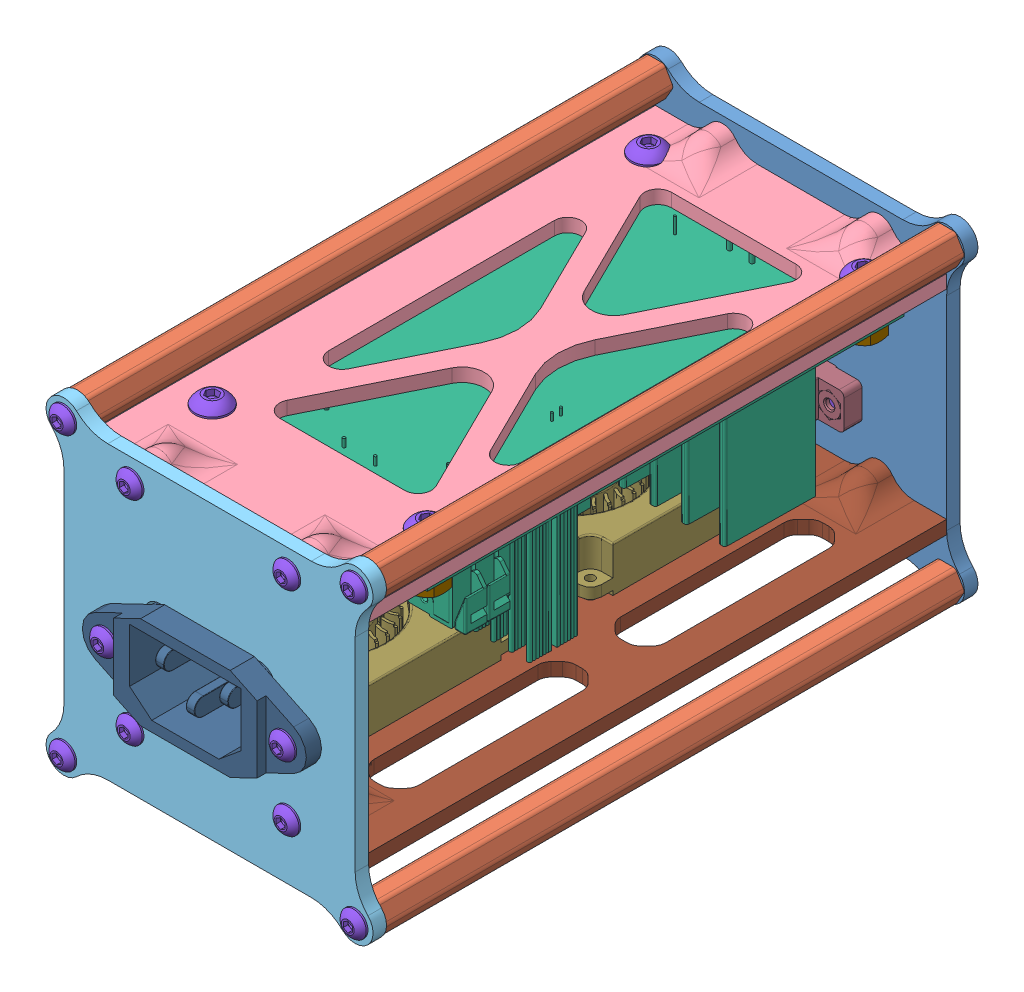
SolidWorks assembly ASM-box-changer-power, configuration По умолчанию. Lengths in mm.
Overall size (73 73 142.05).
63 component instances, 13 part files, 116 mates.
Components (placement in the parent):
- 65-65-3-1: 65-65-3 [По умолчанию] at origin size (73 73 3)
- stoyka-7-129-1: stoyka-7-129 [По умолчанию] at (-32.5 -32.5 3) size (7.77 7 129)
- M3 insert nut.step-1: M3 insert nut.step [По умолчанию] at (-32.5 -32.5 6.1) size (4.49 4.48 6.21)
- M3 insert nut.step-2: M3 insert nut.step [По умолчанию] at (-32.5 -32.5 128.9) size (4.49 4.48 6.21)
- M3 insert nut.step-3: M3 insert nut.step [По умолчанию] at (-32.5 32.5 128.9) size (4.49 4.48 6.21)
- M3 insert nut.step-4: M3 insert nut.step [По умолчанию] at (32.5 -32.5 128.9) size (4.49 4.48 6.21)
- M3 insert nut.step-5: M3 insert nut.step [По умолчанию] at (32.5 32.5 128.9) size (4.49 4.48 6.21)
- M3 insert nut.step-6: M3 insert nut.step [По умолчанию] at (-32.5 32.5 6.1) size (4.49 4.48 6.21)
- M3 insert nut.step-7: M3 insert nut.step [По умолчанию] at (32.5 -32.5 6.1) size (4.49 4.48 6.21)
- M3 insert nut.step-8: M3 insert nut.step [По умолчанию] at (32.5 32.5 6.1) size (4.49 4.48 6.21)
- stoyka-7-129-2: stoyka-7-129 [По умолчанию] at (-32.5 32.5 3) size (7.77 7 129)
- stoyka-7-129-3: stoyka-7-129 [По умолчанию] at (32.5 -32.5 3) size (7.77 7 129)
- stoyka-7-129-4: stoyka-7-129 [По умолчанию] at (32.5 32.5 3) size (7.77 7 129)
- level-0-1: level-0 [По умолчанию] at (0 27 67.5) x (0 0 1) z (0 -1 0) size (129 65 7)
- M3 insert nut.step-9: M3 insert nut.step [По умолчанию] at (-17.5 27.5 6.1) size (4.49 4.48 6.21)
- M3 insert nut.step-10: M3 insert nut.step [По умолчанию] at (17.5 27.5 6.1) size (4.49 4.48 6.21)
- M3 insert nut.step-11: M3 insert nut.step [По умолчанию] at (17.5 27.5 128.9) size (4.49 4.48 6.21)
- M3 insert nut.step-12: M3 insert nut.step [По умолчанию] at (-17.5 27.5 128.9) size (4.49 4.48 6.21)
- 65-65-3-down-1: 65-65-3-down [По умолчанию] at (0 0 132) size (73 73 3)
- WX-DC2412-1: WX-DC2412 [По умолчанию] at (0 21 61.7) x (0 0 -1) z (0 -1 0) size (106.4 57 32.5)
- 4-8-3-1: 4-8-3 [По умолчанию] at (24 21 110.4) x (0.995679 0 0.09286) z (-0.09286 0 0.995679) size (8 3 8)
- 4-8-3-2: 4-8-3 [По умолчанию] at (24 21 13) size (8 3 8)
- 4-8-3-3: 4-8-3 [По умолчанию] at (-24 21 110.4) size (8 3 8)
- 4-8-3-4: 4-8-3 [По умолчанию] at (-24 21 13) size (8 3 8)
- socket button head screw_iso-1: socket button head screw_iso [ISO 7380 - M3 x 8 - 8N] at (17.5 27.5 136.65) x (0 0 -1) z (1 0 0) size (9.65 5.7 5.7)
- socket button head screw_iso-2: socket button head screw_iso [ISO 7380 - M3 x 8 - 8N] at (-17.5 27.5 136.65) x (0 0 -1) z (1 0 0) size (9.65 5.7 5.7)
- socket button head screw_iso-3: socket button head screw_iso [ISO 7380 - M3 x 8 - 8N] at (-32.5 32.5 136.65) x (0 0 -1) z (1 0 0) size (9.65 5.7 5.7)
- socket button head screw_iso-4: socket button head screw_iso [ISO 7380 - M3 x 8 - 8N] at (32.5 32.5 136.65) x (0 0 -1) z (1 0 0) size (9.65 5.7 5.7)
- socket button head screw_iso-5: socket button head screw_iso [ISO 7380 - M3 x 8 - 8N] at (17.5 27.5 -1.65) x (0 0 1) z (-1 0 0) size (9.65 5.7 5.7)
- socket button head screw_iso-6: socket button head screw_iso [ISO 7380 - M3 x 8 - 8N] at (32.5 32.5 -1.65) x (0 0 1) z (-1 0 0) size (9.65 5.7 5.7)
- socket button head screw_iso-7: socket button head screw_iso [ISO 7380 - M3 x 8 - 8N] at (-17.5 27.5 -1.65) x (0 0 1) z (-1 0 0) size (9.65 5.7 5.7)
- socket button head screw_iso-8: socket button head screw_iso [ISO 7380 - M3 x 8 - 8N] at (-32.5 32.5 -1.65) x (0 0 1) z (-1 0 0) size (9.65 5.7 5.7)
- socket button head screw_iso-9: socket button head screw_iso [ISO 7380 - M4 x 12 - 12N] at (24 29.2 110.4) x (0 -1 0) z (0 0 1) size (14.2 7.6 7.6)
- socket button head screw_iso-10: socket button head screw_iso [ISO 7380 - M4 x 12 - 12N] at (24 29.2 13) x (0 -1 0) z (0 0 1) size (14.2 7.6 7.6)
- socket button head screw_iso-11: socket button head screw_iso [ISO 7380 - M4 x 12 - 12N] at (-24 29.2 13) x (0 -1 0) z (0 0 1) size (14.2 7.6 7.6)
- socket button head screw_iso-12: socket button head screw_iso [ISO 7380 - M4 x 12 - 12N] at (-24 29.2 110.4) x (0 -1 0) z (0 0 1) size (14.2 7.6 7.6)
- hex nut style 1 gradeab_iso-1: hex nut style 1 gradeab_iso [ISO - 4032 - M4 - D - N] at (24 16.3 110.4) x (1 0 0) z (0 -1 0) size (7 8.08 3.2)
- hex nut style 1 gradeab_iso-2: hex nut style 1 gradeab_iso [ISO - 4032 - M4 - D - N] at (24 16.28 13) x (1 0 0) z (0 -1 0) size (7 8.08 3.2)
- hex nut style 1 gradeab_iso-3: hex nut style 1 gradeab_iso [ISO - 4032 - M4 - D - N] at (-24 16.3 13) x (1 0 0) z (0 -1 0) size (7 8.08 3.2)
- hex nut style 1 gradeab_iso-4: hex nut style 1 gradeab_iso [ISO - 4032 - M4 - D - N] at (-24 16.28 110.4) x (1 0 0) z (0 -1 0) size (7 8.08 3.2)
- interlock.stp-1: interlock.stp [По умолчанию] at (0 -2.6153 135) size (50 20.7 27.56)
- level-1-1: level-1 [По умолчанию] at (0 -20.5 67.5) x (0 0 1) z (0 -1 0) size (129 65 7)
- 4010 turbo fan v3-1: 4010 turbo fan v3 [По умолчанию] at (-10 -20.5 40) x (1 0 0) z (0 1 0) size (40 40 10)
- 4010 turbo fan v3-2: 4010 turbo fan v3 [По умолчанию] at (-10 -20.5 95) x (1 0 0) z (0 1 0) size (40 40 10)
- M3 insert nut.step-13: M3 insert nut.step [По умолчанию] at (-17.5 -20 128.9) size (4.49 4.48 6.21)
- M3 insert nut.step-14: M3 insert nut.step [По умолчанию] at (17.5 -20 128.9) size (4.49 4.48 6.21)
- M3 insert nut.step-15: M3 insert nut.step [По умолчанию] at (-17.5 -20 6.1) size (4.49 4.48 6.21)
- M3 insert nut.step-16: M3 insert nut.step [По умолчанию] at (17.5 -20 6.1) size (4.49 4.48 6.21)
- socket button head screw_iso-13: socket button head screw_iso [ISO 7380 - M3 x 12 - 12N] at (-20 -2.6153 140.05) x (0 0 -1) z (1 0 0) size (13.65 5.7 5.7)
- socket button head screw_iso-14: socket button head screw_iso [ISO 7380 - M3 x 12 - 12N] at (20 -2.6153 140.05) x (0 0 -1) z (1 0 0) size (13.65 5.7 5.7)
- socket button head screw_iso-17: socket button head screw_iso [ISO 7380 - M3 x 8 - 8N] at (-17.5 -20 136.65) x (0 0 -1) z (1 0 0) size (9.65 5.7 5.7)
- socket button head screw_iso-18: socket button head screw_iso [ISO 7380 - M3 x 8 - 8N] at (17.5 -20 136.65) x (0 0 -1) z (1 0 0) size (9.65 5.7 5.7)
- socket button head screw_iso-19: socket button head screw_iso [ISO 7380 - M3 x 8 - 8N] at (-32.5 -32.5 136.65) x (0 0 -1) z (1 0 0) size (9.65 5.7 5.7)
- socket button head screw_iso-20: socket button head screw_iso [ISO 7380 - M3 x 8 - 8N] at (32.5 -32.5 136.65) x (0 0 -1) z (1 0 0) size (9.65 5.7 5.7)
- socket button head screw_iso-21: socket button head screw_iso [ISO 7380 - M3 x 8 - 8N] at (-32.5 -32.5 -1.65) x (0 0 1) z (-1 0 0) size (9.65 5.7 5.7)
- socket button head screw_iso-22: socket button head screw_iso [ISO 7380 - M3 x 8 - 8N] at (32.5 -32.5 -1.65) x (0 0 1) z (-1 0 0) size (9.65 5.7 5.7)
- hex nut style 1 gradeab_iso-5: hex nut style 1 gradeab_iso [ISO - 4032 - M3 - D - N] at (-20 -2.6153 129.6) x (0.923728 0.383049 0) z (0 0 -1) size (5.5 6.35 2.4)
- hex nut style 1 gradeab_iso-6: hex nut style 1 gradeab_iso [ISO - 4032 - M3 - D - N] at (20 -2.6153 129.6) x (0.923728 0.383049 0) z (0 0 -1) size (5.5 6.35 2.4)
- socket button head screw_iso-23: socket button head screw_iso [ISO 7380 - M3 x 8 - 8N] at (17.5 -20 -1.65) x (0 0 1) z (-1 0 0) size (9.65 5.7 5.7)
- socket button head screw_iso-24: socket button head screw_iso [ISO 7380 - M3 x 8 - 8N] at (-17.5 -20 -1.65) x (0 0 1) z (-1 0 0) size (9.65 5.7 5.7)
- XT60E-M-1: XT60E-M [00] at (0 -7.5 0) x (1 0 0) z (0 -1 0) size (27.2 16.65 9.1)
- socket button head screw_iso-27: socket button head screw_iso [ISO 7380 - M3 x 6 - 6N] at (10.3 -7.5 -1.65) x (0 0 1) z (-1 0 0) size (7.65 5.7 5.7)
- socket button head screw_iso-28: socket button head screw_iso [ISO 7380 - M3 x 6 - 6N] at (-10.3 -7.5 -1.65) x (0 0 1) z (-1 0 0) size (7.65 5.7 5.7)
Mates (geometry in assembly coordinates):
- Концентричный1: concentric anti-aligned: cylinder of 65-65-3-1 through (-32.5 -32.5 3) axis (0 0 -1) radius 1.625; cylinder of stoyka-7-129-1 through (-32.5 -32.5 126) axis (0 0 1) radius 2.25
- Параллельность1: parallel aligned: plane of 65-65-3-1 through (0 -32.5 3) normal (0 -1 0); plane of stoyka-7-129-1 through (-33.9434 -36 132) normal (0 -1 0)
- Концентричный2: concentric aligned: cylinder of stoyka-7-129-1 through (-32.5 -32.5 9) axis (0 0 -1) radius 2.25; cylinder of M3 insert nut.step-1 through (-32.5 -32.5 9.2) axis (0 0 -1) radius 2
- Совпадение2: coincident aligned: plane of stoyka-7-129-1 through (-35.3868 -32.5 3) normal (0 0 -1); plane of M3 insert nut.step-1 through (-32.5 -32.5 3) normal (0 0 -1)
- Концентричный3: concentric anti-aligned: cylinder of stoyka-7-129-1 through (-32.5 -32.5 126) axis (0 0 1) radius 2.25; cylinder of M3 insert nut.step-2 through (-32.5 -32.5 132) axis (0 0 -1) radius 2
- Совпадение3: coincident aligned: plane of stoyka-7-129-1 through (-35.3868 -32.5 132) normal (0 0 1); plane of M3 insert nut.step-2 through (-32.5 -32.5 132) normal (0 0 1)
- Совпадение4: coincident anti-aligned: plane of 65-65-3-1 through (0 0 3) normal (0 0 1); plane of stoyka-7-129-1 through (-35.3868 -32.5 3) normal (0 0 -1)
- Концентричный4: concentric aligned: cylinder of level-0-1 through (-17.5 27.5 9) axis (0 0 -1) radius 2; cylinder of M3 insert nut.step-9 through (-17.5 27.5 9.2) axis (0 0 -1) radius 2
- Совпадение5: coincident aligned: plane of level-0-1 through (32.5 24 3) normal (0 0 -1); plane of M3 insert nut.step-9 through (-17.5 27.5 3) normal (0 0 -1)
- Концентричный5: concentric aligned: cylinder of level-0-1 through (17.5 27.5 9) axis (0 0 -1) radius 2; cylinder of M3 insert nut.step-10 through (17.5 27.5 9.2) axis (0 0 -1) radius 2
- Совпадение6: coincident aligned: plane of level-0-1 through (32.5 24 3) normal (0 0 -1); plane of M3 insert nut.step-10 through (17.5 27.5 3) normal (0 0 -1)
- Концентричный6: concentric anti-aligned: cylinder of level-0-1 through (17.5 27.5 126) axis (0 0 1) radius 2; cylinder of M3 insert nut.step-11 through (17.5 27.5 132) axis (0 0 -1) radius 2
- Совпадение8: coincident aligned: plane of level-0-1 through (32.5 24 132) normal (0 0 1); plane of M3 insert nut.step-11 through (17.5 27.5 132) normal (0 0 1)
- Концентричный7: concentric anti-aligned: cylinder of level-0-1 through (-17.5 27.5 126) axis (0 0 1) radius 2; cylinder of M3 insert nut.step-12 through (-17.5 27.5 132) axis (0 0 -1) radius 2
- Совпадение9: coincident aligned: plane of level-0-1 through (32.5 24 132) normal (0 0 1); plane of M3 insert nut.step-12 through (-17.5 27.5 132) normal (0 0 1)
- Совпадение10: coincident aligned: axis of M3 insert nut.step-5 through (32.5 32.5 130.25) axis (0 0 -1); line of 65-65-3-down-1 through (32.5 32.5 135) axis (0 0 -1)
- Параллельность2: parallel aligned: plane of 65-65-3-1 through (0 32.5 3) normal (0 1 0); plane of 65-65-3-down-1 through (0 32.5 135) normal (0 1 0)
- Совпадение12: coincident anti-aligned: plane of stoyka-7-129-4 through (29.6132 32.5 132) normal (0 0 1); plane of 65-65-3-down-1 through (0 0 132) normal (0 0 -1)
- Совпадение13: coincident anti-aligned: line of 65-65-3-1 through (17.5 27.5 3) axis (0 0 -1); line of M3 insert nut.step-10 through (17.5 27.5 3.0576) axis (0 0 1)
- Совпадение14: coincident aligned: line of 65-65-3-1 through (-17.5 27.5 3) axis (0 0 -1); line of level-0-1 through (-17.5 27.5 6.2156) axis (0 0 -1)
- Совпадение15: coincident anti-aligned: plane of 65-65-3-1 through (0 0 3) normal (0 0 1); plane of level-0-1 through (32.5 24 3) normal (0 0 -1)
- Концентричный8: concentric anti-aligned: cylinder of level-0-1 through (24 34 13) axis (0 -1 0) radius 2.25; cylinder of WX-DC2412-1 through (24 19.5 13) axis (0 1 0) radius 2
- Концентричный9: concentric aligned: cylinder of level-0-1 through (24 34 110.4) axis (0 -1 0) radius 2.25; cylinder of WX-DC2412-1 through (24 19.5 110.4) axis (0 -1 0) radius 2
- Концентричный10: concentric aligned: cylinder of level-0-1 through (24 34 13) axis (0 -1 0) radius 2.25; cylinder of 4-8-3-2 through (24 24 13) axis (0 -1 0) radius 2.25
- Концентричный11: concentric anti-aligned: cylinder of WX-DC2412-1 through (24 19.5 13) axis (0 1 0) radius 2; cylinder of 4-8-3-2 through (24 24 13) axis (0 -1 0) radius 2.25
- Совпадение16: coincident anti-aligned: plane of WX-DC2412-1 through (0 21 61.7) normal (0 1 0); plane of 4-8-3-2 through (24 21 13) normal (0 -1 0)
- Концентричный12: concentric anti-aligned: cylinder of WX-DC2412-1 through (24 19.5 110.4) axis (0 -1 0) radius 2; circle of 4-8-3-1
- Совпадение17: coincident anti-aligned: plane of WX-DC2412-1 through (0 21 61.7) normal (0 1 0); plane of 4-8-3-1 through (24 21 110.4) normal (0 -1 0)
- Концентричный13: concentric aligned: cylinder of level-0-1 through (-24 34 110.4) axis (0 -1 0) radius 2.25; cylinder of 4-8-3-3 through (-24 24 110.4) axis (0 -1 0) radius 2.25
- Совпадение18: coincident anti-aligned: plane of WX-DC2412-1 through (0 21 61.7) normal (0 1 0); plane of 4-8-3-3 through (-24 21 110.4) normal (0 -1 0)
- Концентричный14: concentric aligned: cylinder of WX-DC2412-1 through (-24 19.5 13) axis (0 -1 0) radius 2; cylinder of 4-8-3-4 through (-24 24 13) axis (0 -1 0) radius 2.25
- Совпадение19: coincident anti-aligned: plane of WX-DC2412-1 through (0 21 61.7) normal (0 1 0); plane of 4-8-3-4 through (-24 21 13) normal (0 -1 0)
- Совпадение20: coincident anti-aligned: plane of level-0-1 through (0 24 67.5) normal (0 -1 0); plane of 4-8-3-4 through (-24 24 13) normal (0 1 0)
- Концентричный15: concentric anti-aligned: cylinder of 65-65-3-down-1 through (17.5 27.5 142) axis (0 0 -1) radius 1.75; cylinder of socket button head screw_iso-1 through (17.5 27.5 136.65) axis (0 0 1) radius 2.85
- Совпадение21: coincident anti-aligned: plane of 65-65-3-down-1 through (0 0 135) normal (0 0 1); plane of socket button head screw_iso-1 through (17.5 29 135) normal (0 0 -1)
- Концентричный16: concentric anti-aligned: cylinder of 65-65-3-down-1 through (-17.5 27.5 142) axis (0 0 -1) radius 1.75; cylinder of socket button head screw_iso-2 through (-17.5 27.5 136.65) axis (0 0 1) radius 2.85
- Совпадение22: coincident anti-aligned: plane of 65-65-3-down-1 through (0 0 135) normal (0 0 1); plane of socket button head screw_iso-2 through (-17.5 29 135) normal (0 0 -1)
- Концентричный17: concentric anti-aligned: cylinder of 65-65-3-down-1 through (-32.5 32.5 135) axis (0 0 -1) radius 1.625; cylinder of socket button head screw_iso-3 through (-32.5 32.5 136.65) axis (0 0 1) radius 2.85
- Совпадение23: coincident anti-aligned: plane of 65-65-3-down-1 through (0 0 135) normal (0 0 1); plane of socket button head screw_iso-3 through (-32.5 34 135) normal (0 0 -1)
- Концентричный18: concentric anti-aligned: cylinder of 65-65-3-down-1 through (32.5 32.5 135) axis (0 0 -1) radius 4; cylinder of socket button head screw_iso-4 through (32.5 32.5 136.65) axis (0 0 1) radius 2.85
- Совпадение24: coincident anti-aligned: plane of 65-65-3-down-1 through (0 0 135) normal (0 0 1); plane of socket button head screw_iso-4 through (32.5 34 135) normal (0 0 -1)
- Концентричный19: concentric aligned: cylinder of 65-65-3-1 through (17.5 27.5 10) axis (0 0 -1) radius 1.75; cylinder of socket button head screw_iso-5 through (17.5 27.5 -1.65) axis (0 0 -1) radius 2.85
- Совпадение25: coincident anti-aligned: plane of 65-65-3-1 through (0 0 0) normal (0 0 -1); plane of socket button head screw_iso-5 through (17.5 29 0) normal (0 0 1)
- Концентричный20: concentric aligned: cylinder of 65-65-3-1 through (32.5 32.5 3) axis (0 0 -1) radius 1.625; cylinder of socket button head screw_iso-6 through (32.5 32.5 -1.65) axis (0 0 -1) radius 2.85
- Совпадение26: coincident anti-aligned: plane of 65-65-3-1 through (0 0 0) normal (0 0 -1); plane of socket button head screw_iso-6 through (32.5 34 0) normal (0 0 1)
- Концентричный21: concentric aligned: cylinder of 65-65-3-1 through (-17.5 27.5 10) axis (0 0 -1) radius 1.75; cylinder of socket button head screw_iso-7 through (-17.5 27.5 -1.65) axis (0 0 -1) radius 2.85
- Совпадение27: coincident anti-aligned: plane of 65-65-3-1 through (0 0 0) normal (0 0 -1); plane of socket button head screw_iso-7 through (-17.5 29 0) normal (0 0 1)
- Концентричный22: concentric aligned: cylinder of 65-65-3-1 through (-32.5 32.5 3) axis (0 0 -1) radius 1.625; cylinder of socket button head screw_iso-8 through (-32.5 32.5 -1.65) axis (0 0 -1) radius 2.85
- Совпадение28: coincident anti-aligned: plane of 65-65-3-1 through (0 0 0) normal (0 0 -1); plane of socket button head screw_iso-8 through (-32.5 34 0) normal (0 0 1)
- Концентричный23: concentric anti-aligned: cylinder of level-0-1 through (24 34 110.4) axis (0 -1 0) radius 2.25; cylinder of socket button head screw_iso-9 through (24 29.2 110.4) axis (0 1 0) radius 3.8
- Совпадение29: coincident anti-aligned: plane of level-0-1 through (0 27 67.5) normal (0 1 0); plane of socket button head screw_iso-9 through (26 27 110.4) normal (0 -1 0)
- Концентричный24: concentric anti-aligned: cylinder of level-0-1 through (24 34 13) axis (0 -1 0) radius 2.25; cylinder of socket button head screw_iso-10 through (24 29.2 13) axis (0 1 0) radius 3.8
- Совпадение30: coincident anti-aligned: plane of level-0-1 through (0 27 67.5) normal (0 1 0); plane of socket button head screw_iso-10 through (26 27 13) normal (0 -1 0)
- Концентричный25: concentric anti-aligned: cylinder of level-0-1 through (-24 34 13) axis (0 -1 0) radius 2.25; cylinder of socket button head screw_iso-11 through (-24 29.2 13) axis (0 1 0) radius 3.8
- Совпадение31: coincident anti-aligned: plane of level-0-1 through (0 27 67.5) normal (0 1 0); plane of socket button head screw_iso-11 through (-22 27 13) normal (0 -1 0)
- Концентричный26: concentric anti-aligned: cylinder of level-0-1 through (-24 34 110.4) axis (0 -1 0) radius 2.25; cylinder of socket button head screw_iso-12 through (-24 29.2 110.4) axis (0 1 0) radius 3.8
- Совпадение32: coincident anti-aligned: plane of level-0-1 through (0 27 67.5) normal (0 1 0); plane of socket button head screw_iso-12 through (-22 27 110.4) normal (0 -1 0)
- Концентричный27: concentric aligned: cylinder of WX-DC2412-1 through (24 19.5 110.4) axis (0 -1 0) radius 2; cylinder of hex nut style 1 gradeab_iso-1 through (24 41.3375 110.4) axis (0 -1 0) radius 2
- Совпадение33: coincident anti-aligned: plane of WX-DC2412-1 through (0 19.5 61.7) normal (0 -1 0); plane of hex nut style 1 gradeab_iso-1 through (24 19.5 114.4415) normal (0 1 0)
- Концентричный28: concentric aligned: cylinder of WX-DC2412-1 through (24 140.2154 13) axis (0 -1 0) radius 2.15; cylinder of hex nut style 1 gradeab_iso-2 through (24 41.3175 13) axis (0 -1 0) radius 2
- Совпадение34: coincident anti-aligned: plane of WX-DC2412-1 through (0 19.48 61.7) normal (0 -1 0); plane of hex nut style 1 gradeab_iso-2 through (24 19.48 17.0415) normal (0 1 0)
- Концентричный29: concentric aligned: cylinder of WX-DC2412-1 through (-24 19.5 13) axis (0 -1 0) radius 2; cylinder of hex nut style 1 gradeab_iso-3 through (-24 41.3375 13) axis (0 -1 0) radius 2
- Совпадение35: coincident anti-aligned: plane of WX-DC2412-1 through (0 19.5 61.7) normal (0 -1 0); plane of hex nut style 1 gradeab_iso-3 through (-24 19.5 17.0415) normal (0 1 0)
- Концентричный30: concentric aligned: cylinder of WX-DC2412-1 through (-24 140.2154 110.4) axis (0 -1 0) radius 2.15; cylinder of hex nut style 1 gradeab_iso-4 through (-24 41.3175 110.4) axis (0 -1 0) radius 2
- Совпадение36: coincident anti-aligned: plane of WX-DC2412-1 through (0 19.48 61.7) normal (0 -1 0); plane of hex nut style 1 gradeab_iso-4 through (-24 19.48 114.4415) normal (0 1 0)
- Совпадение37: coincident anti-aligned: plane of 65-65-3-down-1 through (0 0 135) normal (0 0 1); plane of interlock.stp-1 through (0 -2.6153 135) normal (0 0 -1)
- Концентричный31: concentric aligned: cylinder of 65-65-3-down-1 through (-20 -2.6153 142) axis (0 0 -1) radius 1.75; cylinder of interlock.stp-1 through (-20 -2.6153 135) axis (0 0 -1) radius 1.5
- Концентричный32: concentric aligned: cylinder of 65-65-3-down-1 through (20 -2.6153 142) axis (0 0 -1) radius 1.75; cylinder of interlock.stp-1 through (20 -2.6153 135) axis (0 0 -1) radius 1.5
- Совпадение38: coincident anti-aligned: plane of 65-65-3-down-1 through (0 0 132) normal (0 0 -1); plane of level-1-1 through (32.5 -23.5 132) normal (0 0 1)
- Совпадение39: coincident aligned: plane of 65-65-3-down-1 through (-32.5 0 135) normal (-1 0 0); plane of level-1-1 through (-32.5 -23.5 3) normal (-1 0 0)
- Концентричный33: concentric anti-aligned: cylinder of level-1-1 through (-27.5 -13.5 22.5) axis (0 -1 0) radius 1.25; cylinder of 4010 turbo fan v3-1 through (-27.5 -19.5 22.5) axis (0 1 0) radius 1
- Концентричный34: concentric anti-aligned: cylinder of level-1-1 through (-27.5 -13.5 57.5) axis (0 -1 0) radius 1.25; cylinder of 4010 turbo fan v3-1 through (-27.5 -19.5 57.5) axis (0 1 0) radius 1
- Совпадение40: coincident anti-aligned: plane of level-1-1 through (0 -20.5 67.5) normal (0 1 0); plane of 4010 turbo fan v3-1 through (-10 -20.5 40) normal (0 -1 0)
- Концентричный35: concentric anti-aligned: cylinder of level-1-1 through (-27.5 -13.5 77.5) axis (0 -1 0) radius 1.25; cylinder of 4010 turbo fan v3-2 through (-27.5 -19.5 77.5) axis (0 1 0) radius 1
- Концентричный36: concentric anti-aligned: cylinder of level-1-1 through (-27.5 -13.5 112.5) axis (0 -1 0) radius 1.25; cylinder of 4010 turbo fan v3-2 through (-27.5 -19.5 112.5) axis (0 1 0) radius 1
- Совпадение41: coincident anti-aligned: plane of level-1-1 through (0 -20.5 67.5) normal (0 1 0); plane of 4010 turbo fan v3-2 through (-10 -20.5 95) normal (0 -1 0)
- Концентричный37: concentric anti-aligned: cylinder of level-1-1 through (-17.5 -20 126) axis (0 0 1) radius 2; cylinder of M3 insert nut.step-13 through (-17.5 -20 132) axis (0 0 -1) radius 2
- Совпадение42: coincident aligned: plane of level-1-1 through (32.5 -23.5 132) normal (0 0 1); plane of M3 insert nut.step-13 through (-17.5 -20 132) normal (0 0 1)
- Концентричный38: concentric anti-aligned: cylinder of level-1-1 through (17.5 -20 126) axis (0 0 1) radius 2; cylinder of M3 insert nut.step-14 through (17.5 -20 132) axis (0 0 -1) radius 2
- Совпадение43: coincident aligned: plane of level-1-1 through (32.5 -23.5 132) normal (0 0 1); circle of M3 insert nut.step-14
- Концентричный39: concentric aligned: cylinder of level-1-1 through (-17.5 -20 9) axis (0 0 -1) radius 2; cylinder of M3 insert nut.step-15 through (-17.5 -20 9.2) axis (0 0 -1) radius 2
- Совпадение44: coincident aligned: plane of level-1-1 through (32.5 -23.5 3) normal (0 0 -1); plane of M3 insert nut.step-15 through (-17.5 -20 3) normal (0 0 -1)
- Концентричный40: concentric aligned: cylinder of level-1-1 through (17.5 -20 9) axis (0 0 -1) radius 2; cylinder of M3 insert nut.step-16 through (17.5 -20 9.2) axis (0 0 -1) radius 2
- Совпадение45: coincident aligned: plane of level-1-1 through (32.5 -23.5 3) normal (0 0 -1); plane of M3 insert nut.step-16 through (17.5 -20 3) normal (0 0 -1)
- Концентричный41: concentric aligned: cylinder of 65-65-3-down-1 through (-17.5 -20 125) axis (0 0 1) radius 1.75; cylinder of M3 insert nut.step-13 through (-17.5 -20 132) axis (0 0 1) radius 1.25
- Концентричный42: concentric anti-aligned: cylinder of interlock.stp-1 through (-20 -2.6153 135) axis (0 0 -1) radius 1.5; cylinder of socket button head screw_iso-13 through (-20 -2.6153 140.05) axis (0 0 1) radius 2.85
- Совпадение46: coincident anti-aligned: plane of interlock.stp-1 through (0 -2.6153 138.4) normal (0 0 1); plane of socket button head screw_iso-13 through (-20 -1.1153 138.4) normal (0 0 -1)
- Концентричный43: concentric anti-aligned: cylinder of interlock.stp-1 through (20 -2.6153 135) axis (0 0 -1) radius 1.5; cylinder of socket button head screw_iso-14 through (20 -2.6153 140.05) axis (0 0 1) radius 2.85
- Совпадение47: coincident anti-aligned: plane of interlock.stp-1 through (0 -2.6153 138.4) normal (0 0 1); plane of socket button head screw_iso-14 through (20 -1.1153 138.4) normal (0 0 -1)
- Концентричный46: concentric aligned: cylinder of 65-65-3-down-1 through (-17.5 -20 125) axis (0 0 1) radius 1.75; cylinder of socket button head screw_iso-17 through (-17.5 -20 136.65) axis (0 0 1) radius 2.85
- Совпадение48: coincident anti-aligned: plane of 65-65-3-down-1 through (0 0 135) normal (0 0 1); plane of socket button head screw_iso-17 through (-17.5 -18.5 135) normal (0 0 -1)
- Концентричный47: concentric aligned: cylinder of 65-65-3-down-1 through (17.5 -20 125) axis (0 0 1) radius 1.75; cylinder of socket button head screw_iso-18 through (17.5 -20 136.65) axis (0 0 1) radius 2.85
- Совпадение49: coincident anti-aligned: plane of 65-65-3-down-1 through (0 0 135) normal (0 0 1); plane of socket button head screw_iso-18 through (17.5 -18.5 135) normal (0 0 -1)
- Концентричный48: concentric anti-aligned: cylinder of 65-65-3-down-1 through (-32.5 -32.5 135) axis (0 0 -1) radius 1.625; cylinder of socket button head screw_iso-19 through (-32.5 -32.5 136.65) axis (0 0 1) radius 2.85
- Совпадение50: coincident anti-aligned: plane of 65-65-3-down-1 through (0 0 135) normal (0 0 1); plane of socket button head screw_iso-19 through (-32.5 -31 135) normal (0 0 -1)
- Концентричный49: concentric anti-aligned: cylinder of 65-65-3-down-1 through (32.5 -32.5 135) axis (0 0 -1) radius 1.625; cylinder of socket button head screw_iso-20 through (32.5 -32.5 136.65) axis (0 0 1) radius 2.85
- Совпадение51: coincident anti-aligned: plane of 65-65-3-down-1 through (0 0 135) normal (0 0 1); plane of socket button head screw_iso-20 through (32.5 -31 135) normal (0 0 -1)
- Концентричный50: concentric aligned: cylinder of 65-65-3-1 through (-32.5 -32.5 3) axis (0 0 -1) radius 1.625; cylinder of socket button head screw_iso-21 through (-32.5 -32.5 -1.65) axis (0 0 -1) radius 2.85
- Совпадение52: coincident anti-aligned: plane of 65-65-3-1 through (0 0 0) normal (0 0 -1); plane of socket button head screw_iso-21 through (-32.5 -31 0) normal (0 0 1)
- Концентричный51: concentric aligned: cylinder of 65-65-3-1 through (32.5 -32.5 3) axis (0 0 -1) radius 1.625; cylinder of socket button head screw_iso-22 through (32.5 -32.5 -1.65) axis (0 0 -1) radius 2.85
- Совпадение53: coincident anti-aligned: plane of 65-65-3-1 through (0 0 0) normal (0 0 -1); plane of socket button head screw_iso-22 through (32.5 -31 0) normal (0 0 1)
- Концентричный52: concentric aligned: cylinder of 65-65-3-down-1 through (-20 -2.6153 142) axis (0 0 -1) radius 1.75; cylinder of hex nut style 1 gradeab_iso-5 through (-20 -2.6153 154.6375) axis (0 0 -1) radius 1.5
- Совпадение54: coincident anti-aligned: plane of 65-65-3-down-1 through (0 0 132) normal (0 0 -1); plane of hex nut style 1 gradeab_iso-5 through (-18.7837 -5.5485 132) normal (0 0 1)
- Концентричный53: concentric aligned: cylinder of 65-65-3-down-1 through (20 -2.6153 142) axis (0 0 -1) radius 1.75; cylinder of hex nut style 1 gradeab_iso-6 through (20 -2.6153 154.6375) axis (0 0 -1) radius 1.5
- Совпадение55: coincident anti-aligned: plane of 65-65-3-down-1 through (0 0 132) normal (0 0 -1); plane of hex nut style 1 gradeab_iso-6 through (21.2163 -5.5485 132) normal (0 0 1)
- Концентричный54: concentric aligned: cylinder of 65-65-3-1 through (17.5 -20 10) axis (0 0 -1) radius 1.75; cylinder of socket button head screw_iso-23 through (17.5 -20 -1.65) axis (0 0 -1) radius 2.85
- Совпадение56: coincident anti-aligned: plane of 65-65-3-1 through (0 0 0) normal (0 0 -1); plane of socket button head screw_iso-23 through (17.5 -18.5 0) normal (0 0 1)
- Концентричный55: concentric aligned: cylinder of 65-65-3-1 through (-17.5 -20 10) axis (0 0 -1) radius 1.75; cylinder of socket button head screw_iso-24 through (-17.5 -20 -1.65) axis (0 0 -1) radius 2.85
- Совпадение57: coincident anti-aligned: plane of 65-65-3-1 through (0 0 0) normal (0 0 -1); plane of socket button head screw_iso-24 through (-17.5 -18.5 0) normal (0 0 1)
- Совпадение58: coincident anti-aligned: plane of 65-65-3-1 through (0 0 3) normal (0 0 1); plane of XT60E-M-1 through (0 -7.5 3) normal (0 0 -1)
- Концентричный56: concentric anti-aligned: cylinder of 65-65-3-1 through (10.3 -7.5 10) axis (0 0 -1) radius 1.75; cylinder of XT60E-M-1 through (10.3 -7.5 3) axis (0 0 1) radius 1.5
- Концентричный57: concentric anti-aligned: cylinder of 65-65-3-1 through (-10.3 -7.5 10) axis (0 0 -1) radius 1.75; cylinder of XT60E-M-1 through (-10.3 -7.5 3) axis (0 0 1) radius 1.5
- Концентричный60: concentric aligned: cylinder of 65-65-3-1 through (10.3 -7.5 10) axis (0 0 -1) radius 1.75; cylinder of socket button head screw_iso-27 through (10.3 -7.5 -1.65) axis (0 0 -1) radius 2.85
- Совпадение60: coincident anti-aligned: plane of 65-65-3-1 through (0 0 0) normal (0 0 -1); plane of socket button head screw_iso-27 through (10.3 -6 0) normal (0 0 1)
- Концентричный61: concentric aligned: cylinder of 65-65-3-1 through (-10.3 -7.5 10) axis (0 0 -1) radius 1.75; cylinder of socket button head screw_iso-28 through (-10.3 -7.5 -1.65) axis (0 0 -1) radius 2.85
- Совпадение61: coincident anti-aligned: plane of 65-65-3-1 through (0 0 0) normal (0 0 -1); plane of socket button head screw_iso-28 through (-10.3 -6 0) normal (0 0 1)
